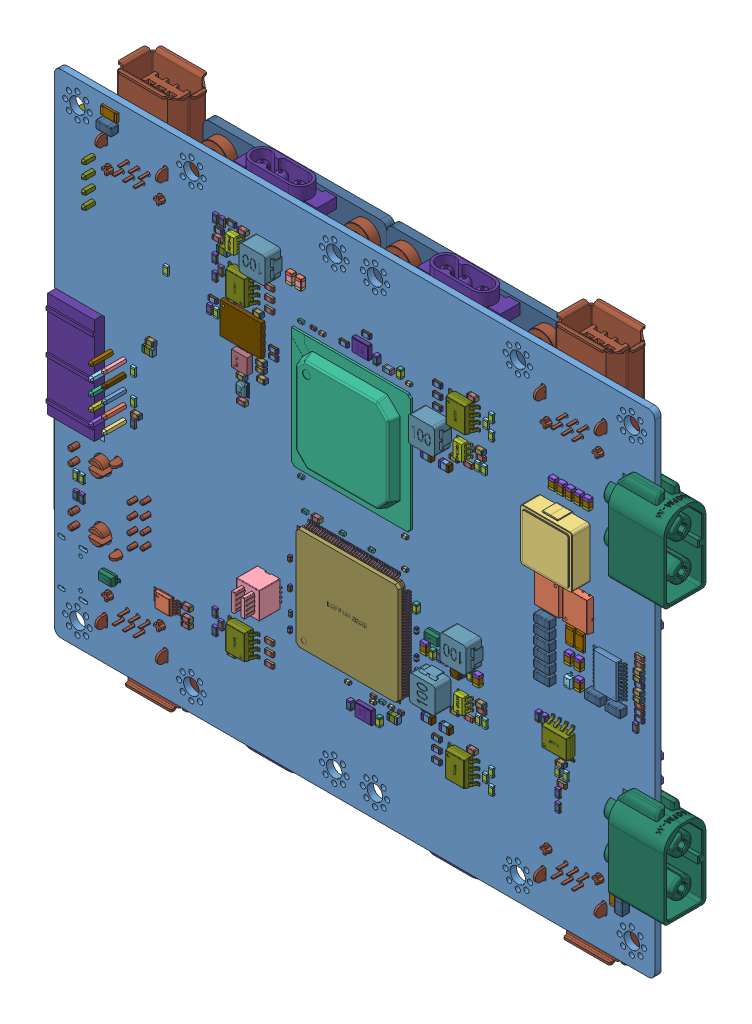
SolidWorks assembly Mother  Board, configuration 默认. Lengths in mm. (continued)
Components (placement in the parent): (continued)
- Mother  Board.step-1: Mother  Board.step [默认] at origin size (122.6 102.08 21) (continued)
  - Free-Models.step-1: Free-Models.step [默认] at origin size (70.87 98.07 8.62) (continued)
    - Driver_Board.step-2: Driver_Board.step [默认] at (84.963 86.106 -6.2) x (-1 0 0) z (0 0 1) size (35.43 49.03 8.62) (continued)
      - C19-1.step-1: C19-1.step [默认] at origin size (0.8 1.6 0.8) (continued)
        - 6547517776.step-1: 6547517776.step [默认] at (25.7809 37.7191 0) x (0 1 0) z (0 0 1) size (1.6 0.8 0.8) (continued)
          - Terminal-24.step-1: Terminal-24.step [默认] at (-0.8 -0.4 0) size (1.6 0.8 0.8) (continued)
            - Open_CASCADE_STEP_translator_6.8_47.1.2-105.step-1: Open_CASCADE_STEP_translator_6.8_47.1.2-105.step [默认] at origin size (0.3 0.8 0.8)
          - Mid_Body-12.step-1: Mid_Body-12.step [默认] at (-0.8 -0.4 0) size (1 0.8 0.8)
            - Open_CASCADE_STEP_translator_6.8_47.2.1-106.step-1: Open_CASCADE_STEP_translator_6.8_47.2.1-106.step [默认] at origin size (1 0.8 0.8)
      - C18-1.step-1: C18-1.step [默认] at origin size (0.8 1.6 0.8)
        - 6547517776.step-1: 6547517776.step [默认] at (24.6379 37.7191 0) x (0 1 0) z (0 0 1) size (1.6 0.8 0.8)
          - Terminal-24.step-1: Terminal-24.step [默认] at (-0.8 -0.4 0) size (1.6 0.8 0.8)
            - Open_CASCADE_STEP_translator_6.8_47.1.1-104.step-1: Open_CASCADE_STEP_translator_6.8_47.1.1-104.step [默认] at origin size (0.3 0.8 0.8)
            - Open_CASCADE_STEP_translator_6.8_47.1.2-105.step-1: Open_CASCADE_STEP_translator_6.8_47.1.2-105.step [默认] at origin size (0.3 0.8 0.8)
          - Mid_Body-12.step-1: Mid_Body-12.step [默认] at (-0.8 -0.4 0) size (1 0.8 0.8)
            - Open_CASCADE_STEP_translator_6.8_47.2.1-106.step-1: Open_CASCADE_STEP_translator_6.8_47.2.1-106.step [默认] at origin size (1 0.8 0.8)
      - C17-1.step-1: C17-1.step [默认] at origin size (1.6 0.8 0.8)
        - 6547515616.step-1: 6547515616.step [默认] at (13.7159 12.9539 0) x (-1 0 0) z (0 0 1) size (1.6 0.8 0.8)
          - Terminal-22.step-1: Terminal-22.step [默认] at (-0.8 -0.4 0) size (1.6 0.8 0.8)
            - Open_CASCADE_STEP_translator_6.8_47.1.1-85.step-1: Open_CASCADE_STEP_translator_6.8_47.1.1-85.step [默认] at origin size (0.3 0.8 0.8)
            - Open_CASCADE_STEP_translator_6.8_47.1.2-86.step-1: Open_CASCADE_STEP_translator_6.8_47.1.2-86.step [默认] at origin size (0.3 0.8 0.8)
          - Mid_Body-10.step-1: Mid_Body-10.step [默认] at (-0.8 -0.4 0) size (1 0.8 0.8)
            - Open_CASCADE_STEP_translator_6.8_47.2.1-87.step-1: Open_CASCADE_STEP_translator_6.8_47.2.1-87.step [默认] at origin size (1 0.8 0.8)
      - C16-1.step-1: C16-1.step [默认] at origin size (0.8 1.6 0.8)
        - 6547516096.step-1: 6547516096.step [默认] at (25.7811 22.2249 0) x (0 -1 0) z (0 0 1) size (1.6 0.8 0.8)
          - Terminal-23.step-1: Terminal-23.step [默认] at (-0.8 -0.4 0) size (1.6 0.8 0.8)
            - Open_CASCADE_STEP_translator_6.8_47.1.1-98.step-1: Open_CASCADE_STEP_translator_6.8_47.1.1-98.step [默认] at origin size (0.3 0.8 0.8)
            - Open_CASCADE_STEP_translator_6.8_47.1.2-99.step-1: Open_CASCADE_STEP_translator_6.8_47.1.2-99.step [默认] at origin size (0.3 0.8 0.8)
          - Mid_Body-11.step-1: Mid_Body-11.step [默认] at (-0.8 -0.4 0) size (1 0.8 0.8)
            - Open_CASCADE_STEP_translator_6.8_47.2.1-100.step-1: Open_CASCADE_STEP_translator_6.8_47.2.1-100.step [默认] at origin size (1 0.8 0.8)
      - C15-1.step-1: C15-1.step [默认] at origin size (0.8 1.6 0.8)
        - 6547517776.step-1: 6547517776.step [默认] at (23.8759 25.6541 0) x (0 1 0) z (0 0 1) size (1.6 0.8 0.8)
          - Terminal-24.step-1: Terminal-24.step [默认] at (-0.8 -0.4 0) size (1.6 0.8 0.8)
            - Open_CASCADE_STEP_translator_6.8_47.1.1-104.step-1: Open_CASCADE_STEP_translator_6.8_47.1.1-104.step [默认] at origin size (0.3 0.8 0.8)
            - Open_CASCADE_STEP_translator_6.8_47.1.2-105.step-1: Open_CASCADE_STEP_translator_6.8_47.1.2-105.step [默认] at origin size (0.3 0.8 0.8)
          - Mid_Body-12.step-1: Mid_Body-12.step [默认] at (-0.8 -0.4 0) size (1 0.8 0.8)
            - Open_CASCADE_STEP_translator_6.8_47.2.1-106.step-1: Open_CASCADE_STEP_translator_6.8_47.2.1-106.step [默认] at origin size (1 0.8 0.8)
      - C14-1.step-1: C14-1.step [默认] at origin size (2.01 1.25 0.94)
        - 6547513136.step-1: 6547513136.step [默认] at (13.7383 23.4725 0) x (-1 0 0) z (0 0 1) size (2.01 1.25 0.94)
          - Fillet1-95.step-1: Fillet1-95.step [默认] at origin size (0.5 1.25 0.94)
          - Fillet2-96.step-1: Fillet2-96.step [默认] at origin size (0.5 1.25 0.94)
          - body2-97.step-1: body2-97.step [默认] at origin size (1.01 1.22 0.92)
      - C13-1.step-1: C13-1.step [默认] at origin size (0.8 1.6 0.8)
        - 6547516096.step-1: 6547516096.step [默认] at (10.8175 24.7425 0) x (0 -1 0) z (0 0 1) size (1.6 0.8 0.8)
          - Terminal-23.step-1: Terminal-23.step [默认] at (-0.8 -0.4 0) size (1.6 0.8 0.8)
            - Open_CASCADE_STEP_translator_6.8_47.1.1-98.step-1: Open_CASCADE_STEP_translator_6.8_47.1.1-98.step [默认] at origin size (0.3 0.8 0.8)
            - Open_CASCADE_STEP_translator_6.8_47.1.2-99.step-1: Open_CASCADE_STEP_translator_6.8_47.1.2-99.step [默认] at origin size (0.3 0.8 0.8)
          - Mid_Body-11.step-1: Mid_Body-11.step [默认] at (-0.8 -0.4 0) size (1 0.8 0.8)
            - Open_CASCADE_STEP_translator_6.8_47.2.1-100.step-1: Open_CASCADE_STEP_translator_6.8_47.2.1-100.step [默认] at origin size (1 0.8 0.8)
      - C12-1.step-1: C12-1.step [默认] at origin size (1.25 2.01 0.94)
        - 6547514896.step-1: 6547514896.step [默认] at (16.4053 31.0126 0) x (0 1 0) z (0 0 1) size (2.01 1.25 0.94)
          - Fillet1-101.step-1: Fillet1-101.step [默认] at origin size (0.5 1.25 0.94)
          - Fillet2-102.step-1: Fillet2-102.step [默认] at origin size (0.5 1.25 0.94)
          - body2-103.step-1: body2-103.step [默认] at origin size (1.01 1.22 0.92)
      - C11-1.step-1: C11-1.step [默认] at origin size (1.6 0.8 0.8)
        - 6547515616.step-1: 6547515616.step [默认] at (27.6859 22.8599 0) x (-1 0 0) z (0 0 1) size (1.6 0.8 0.8)
          - Terminal-22.step-1: Terminal-22.step [默认] at (-0.8 -0.4 0) size (1.6 0.8 0.8)
            - Open_CASCADE_STEP_translator_6.8_47.1.1-85.step-1: Open_CASCADE_STEP_translator_6.8_47.1.1-85.step [默认] at origin size (0.3 0.8 0.8)
            - Open_CASCADE_STEP_translator_6.8_47.1.2-86.step-1: Open_CASCADE_STEP_translator_6.8_47.1.2-86.step [默认] at origin size (0.3 0.8 0.8)
          - Mid_Body-10.step-1: Mid_Body-10.step [默认] at (-0.8 -0.4 0) size (1 0.8 0.8)
            - Open_CASCADE_STEP_translator_6.8_47.2.1-87.step-1: Open_CASCADE_STEP_translator_6.8_47.2.1-87.step [默认] at origin size (1 0.8 0.8)
      - C10-1.step-1: C10-1.step [默认] at origin size (0.8 1.6 0.8)
        - 6547517776.step-1: 6547517776.step [默认] at (-3.1751 37.7191 0) x (0 1 0) z (0 0 1) size (1.6 0.8 0.8)
          - Terminal-24.step-1: Terminal-24.step [默认] at (-0.8 -0.4 0) size (1.6 0.8 0.8)
            - Open_CASCADE_STEP_translator_6.8_47.1.1-104.step-1: Open_CASCADE_STEP_translator_6.8_47.1.1-104.step [默认] at origin size (0.3 0.8 0.8)
            - Open_CASCADE_STEP_translator_6.8_47.1.2-105.step-1: Open_CASCADE_STEP_translator_6.8_47.1.2-105.step [默认] at origin size (0.3 0.8 0.8)
          - Mid_Body-12.step-1: Mid_Body-12.step [默认] at (-0.8 -0.4 0) size (1 0.8 0.8)
            - Open_CASCADE_STEP_translator_6.8_47.2.1-106.step-1: Open_CASCADE_STEP_translator_6.8_47.2.1-106.step [默认] at origin size (1 0.8 0.8)
      - C9-1.step-1: C9-1.step [默认] at origin size (0.8 1.6 0.8)
        - 6547516096.step-1: 6547516096.step [默认] at (-3.1749 22.2249 0) x (0 -1 0) z (0 0 1) size (1.6 0.8 0.8)
          - Terminal-23.step-1: Terminal-23.step [默认] at (-0.8 -0.4 0) size (1.6 0.8 0.8)
            - Open_CASCADE_STEP_translator_6.8_47.1.1-98.step-1: Open_CASCADE_STEP_translator_6.8_47.1.1-98.step [默认] at origin size (0.3 0.8 0.8)
            - Open_CASCADE_STEP_translator_6.8_47.1.2-99.step-1: Open_CASCADE_STEP_translator_6.8_47.1.2-99.step [默认] at origin size (0.3 0.8 0.8)
          - Mid_Body-11.step-1: Mid_Body-11.step [默认] at (-0.8 -0.4 0) size (1 0.8 0.8)
            - Open_CASCADE_STEP_translator_6.8_47.2.1-100.step-1: Open_CASCADE_STEP_translator_6.8_47.2.1-100.step [默认] at origin size (1 0.8 0.8)
      - C8-1.step-1: C8-1.step [默认] at origin size (1.6 0.8 0.8)
        - 6547515616.step-1: 6547515616.step [默认] at (1.1429 16.5099 0) x (-1 0 0) z (0 0 1) size (1.6 0.8 0.8)
          - Terminal-22.step-1: Terminal-22.step [默认] at (-0.8 -0.4 0) size (1.6 0.8 0.8)
            - Open_CASCADE_STEP_translator_6.8_47.1.1-85.step-1: Open_CASCADE_STEP_translator_6.8_47.1.1-85.step [默认] at origin size (0.3 0.8 0.8)
            - Open_CASCADE_STEP_translator_6.8_47.1.2-86.step-1: Open_CASCADE_STEP_translator_6.8_47.1.2-86.step [默认] at origin size (0.3 0.8 0.8)
          - Mid_Body-10.step-1: Mid_Body-10.step [默认] at (-0.8 -0.4 0) size (1 0.8 0.8)
            - Open_CASCADE_STEP_translator_6.8_47.2.1-87.step-1: Open_CASCADE_STEP_translator_6.8_47.2.1-87.step [默认] at origin size (1 0.8 0.8)
      - C7-1.step-1: C7-1.step [默认] at origin size (0.8 1.6 0.8)
        - 6547516096.step-1: 6547516096.step [默认] at (-2.0319 22.2249 0) x (0 -1 0) z (0 0 1) size (1.6 0.8 0.8)
          - Terminal-23.step-1: Terminal-23.step [默认] at (-0.8 -0.4 0) size (1.6 0.8 0.8)
            - Open_CASCADE_STEP_translator_6.8_47.1.1-98.step-1: Open_CASCADE_STEP_translator_6.8_47.1.1-98.step [默认] at origin size (0.3 0.8 0.8)
            - Open_CASCADE_STEP_translator_6.8_47.1.2-99.step-1: Open_CASCADE_STEP_translator_6.8_47.1.2-99.step [默认] at origin size (0.3 0.8 0.8)
          - Mid_Body-11.step-1: Mid_Body-11.step [默认] at (-0.8 -0.4 0) size (1 0.8 0.8)
            - Open_CASCADE_STEP_translator_6.8_47.2.1-100.step-1: Open_CASCADE_STEP_translator_6.8_47.2.1-100.step [默认] at origin size (1 0.8 0.8)
      - C6-1.step-1: C6-1.step [默认] at origin size (0.8 1.6 0.8)
        - 6547517776.step-1: 6547517776.step [默认] at (-2.0321 37.7191 0) x (0 1 0) z (0 0 1) size (1.6 0.8 0.8)
          - Terminal-24.step-1: Terminal-24.step [默认] at (-0.8 -0.4 0) size (1.6 0.8 0.8)
            - Open_CASCADE_STEP_translator_6.8_47.1.1-104.step-1: Open_CASCADE_STEP_translator_6.8_47.1.1-104.step [默认] at origin size (0.3 0.8 0.8)
            - Open_CASCADE_STEP_translator_6.8_47.1.2-105.step-1: Open_CASCADE_STEP_translator_6.8_47.1.2-105.step [默认] at origin size (0.3 0.8 0.8)
          - Mid_Body-12.step-1: Mid_Body-12.step [默认] at (-0.8 -0.4 0) size (1 0.8 0.8)
            - Open_CASCADE_STEP_translator_6.8_47.2.1-106.step-1: Open_CASCADE_STEP_translator_6.8_47.2.1-106.step [默认] at origin size (1 0.8 0.8)
      - C5-1.step-1: C5-1.step [默认] at origin size (1.6 0.8 0.8)
        - 6547515616.step-1: 6547515616.step [默认] at (2.7939 10.6679 0) x (-1 0 0) z (0 0 1) size (1.6 0.8 0.8)
          - Terminal-22.step-1: Terminal-22.step [默认] at (-0.8 -0.4 0) size (1.6 0.8 0.8)
            - Open_CASCADE_STEP_translator_6.8_47.1.1-85.step-1: Open_CASCADE_STEP_translator_6.8_47.1.1-85.step [默认] at origin size (0.3 0.8 0.8)
            - Open_CASCADE_STEP_translator_6.8_47.1.2-86.step-1: Open_CASCADE_STEP_translator_6.8_47.1.2-86.step [默认] at origin size (0.3 0.8 0.8)
          - Mid_Body-10.step-1: Mid_Body-10.step [默认] at (-0.8 -0.4 0) size (1 0.8 0.8)
            - Open_CASCADE_STEP_translator_6.8_47.2.1-87.step-1: Open_CASCADE_STEP_translator_6.8_47.2.1-87.step [默认] at origin size (1 0.8 0.8)
      - C4-1.step-1: C4-1.step [默认] at origin size (1.6 0.8 0.8)
        - 6547515616.step-1: 6547515616.step [默认] at (-0.1271 22.8599 0) x (-1 0 0) z (0 0 1) size (1.6 0.8 0.8)
          - Terminal-22.step-1: Terminal-22.step [默认] at (-0.8 -0.4 0) size (1.6 0.8 0.8)
            - Open_CASCADE_STEP_translator_6.8_47.1.1-85.step-1: Open_CASCADE_STEP_translator_6.8_47.1.1-85.step [默认] at origin size (0.3 0.8 0.8)
            - Open_CASCADE_STEP_translator_6.8_47.1.2-86.step-1: Open_CASCADE_STEP_translator_6.8_47.1.2-86.step [默认] at origin size (0.3 0.8 0.8)
          - Mid_Body-10.step-1: Mid_Body-10.step [默认] at (-0.8 -0.4 0) size (1 0.8 0.8)
            - Open_CASCADE_STEP_translator_6.8_47.2.1-87.step-1: Open_CASCADE_STEP_translator_6.8_47.2.1-87.step [默认] at origin size (1 0.8 0.8)
      - C3-1.step-1: C3-1.step [默认] at origin size (2.01 1.25 0.94)
        - 6547513136.step-1: 6547513136.step [默认] at (6.6263 23.4725 0) x (-1 0 0) z (0 0 1) size (2.01 1.25 0.94)
          - Fillet1-95.step-1: Fillet1-95.step [默认] at origin size (0.5 1.25 0.94)
          - Fillet2-96.step-1: Fillet2-96.step [默认] at origin size (0.5 1.25 0.94)
          - body2-97.step-1: body2-97.step [默认] at origin size (1.01 1.22 0.92)
      - C2-1.step-1: C2-1.step [默认] at origin size (0.8 1.6 0.8)
        - 6547516096.step-1: 6547516096.step [默认] at (3.7055 24.7425 0) x (0 -1 0) z (0 0 1) size (1.6 0.8 0.8)
          - Terminal-23.step-1: Terminal-23.step [默认] at (-0.8 -0.4 0) size (1.6 0.8 0.8)
            - Open_CASCADE_STEP_translator_6.8_47.1.1-98.step-1: Open_CASCADE_STEP_translator_6.8_47.1.1-98.step [默认] at origin size (0.3 0.8 0.8)
            - Open_CASCADE_STEP_translator_6.8_47.1.2-99.step-1: Open_CASCADE_STEP_translator_6.8_47.1.2-99.step [默认] at origin size (0.3 0.8 0.8)
          - Mid_Body-11.step-1: Mid_Body-11.step [默认] at (-0.8 -0.4 0) size (1 0.8 0.8)
            - Open_CASCADE_STEP_translator_6.8_47.2.1-100.step-1: Open_CASCADE_STEP_translator_6.8_47.2.1-100.step [默认] at origin size (1 0.8 0.8)
      - C1.step-1: C1.step [默认] at origin size (1.25 2.01 0.94)
        - 6547514896.step-1: 6547514896.step [默认] at (9.2933 31.0126 0) x (0 1 0) z (0 0 1) size (2.01 1.25 0.94)
          - Fillet1-101.step-1: Fillet1-101.step [默认] at origin size (0.5 1.25 0.94)
          - Fillet2-102.step-1: Fillet2-102.step [默认] at origin size (0.5 1.25 0.94)
          - body2-103.step-1: body2-103.step [默认] at origin size (1.01 1.22 0.92)
    - Driver_Board.step-3: Driver_Board.step [默认] at (57.3933 0 -6.2) x (1 0 0) z (0 0 1) size (35.43 49.03 8.62)
      - Board-1.step-1: Board-1.step [默认] at origin size (35.43 46.99 1.62)
        - Open_CASCADE_STEP_translator_6.8_2.1.1.step-1: Open_CASCADE_STEP_translator_6.8_2.1.1.step [默认] at (0 0 -1.6164) size (35.43 46.99 1.62)
      - R25-1.step-1: R25-1.step [默认] at origin size (0.8 1.6 0.45)
        - 6547515376.step-1: 6547515376.step [默认] at (20.6304 35.5601 0) x (0 1 0) z (0 0 1) size (1.6 0.8 0.45)
          - Terminal-19.step-1: Terminal-19.step [默认] at (-0.8 -0.4 0) size (0.3 0.8 0.45)
            - Open_CASCADE_STEP_translator_6.8_21.2.1-76.step-1: Open_CASCADE_STEP_translator_6.8_21.2.1-76.step [默认] at origin size (0.3 0.8 0.45)
          - Terminal-19.step-2: Terminal-19.step [默认] at (0.8 0.4 0) x (-1 0 0) z (0 0 1) size (0.3 0.8 0.45)
            - Open_CASCADE_STEP_translator_6.8_21.2.1-76.step-1: Open_CASCADE_STEP_translator_6.8_21.2.1-76.step [默认] at origin size (0.3 0.8 0.45)
          - Mid_Body-77.step-1: Mid_Body-77.step [默认] at (-0.8 -0.4 0) size (1.51 0.8 0.36)
          - Mark-78.step-1: Mark-78.step [默认] at (-0.5 -0.4 0.405) size (1 0.8 0.05)
      - R24-1.step-1: R24-1.step [默认] at origin size (1.6 0.8 0.45)
        - 6547516336.step-1: 6547516336.step [默认] at (12.6999 34.9249 0) x (-1 0 0) z (0 0 1) size (1.6 0.8 0.45)
          - Terminal-20.step-1: Terminal-20.step [默认] at (-0.8 -0.4 0) size (0.3 0.8 0.45)
            - Open_CASCADE_STEP_translator_6.8_21.2.1-79.step-1: Open_CASCADE_STEP_translator_6.8_21.2.1-79.step [默认] at origin size (0.3 0.8 0.45)
          - Terminal-20.step-2: Terminal-20.step [默认] at (0.8 0.4 0) x (-1 0 0) z (0 0 1) size (0.3 0.8 0.45)
            - Open_CASCADE_STEP_translator_6.8_21.2.1-79.step-1: Open_CASCADE_STEP_translator_6.8_21.2.1-79.step [默认] at origin size (0.3 0.8 0.45)
          - Mid_Body-80.step-1: Mid_Body-80.step [默认] at (-0.8 -0.4 0) size (1.51 0.8 0.36)
          - Mark-81.step-1: Mark-81.step [默认] at (-0.5 -0.4 0.405) size (1 0.8 0.05)
      - R23-1.step-1: R23-1.step [默认] at origin size (1.6 0.8 0.45)
        - 6547516336.step-1: 6547516336.step [默认] at (5.5879 33.6549 0) x (-1 0 0) z (0 0 1) size (1.6 0.8 0.45)
          - Terminal-20.step-1: Terminal-20.step [默认] at (-0.8 -0.4 0) size (0.3 0.8 0.45)
            - Open_CASCADE_STEP_translator_6.8_21.2.1-79.step-1: Open_CASCADE_STEP_translator_6.8_21.2.1-79.step [默认] at origin size (0.3 0.8 0.45)
          - Terminal-20.step-2: Terminal-20.step [默认] at (0.8 0.4 0) x (-1 0 0) z (0 0 1) size (0.3 0.8 0.45)
            - Open_CASCADE_STEP_translator_6.8_21.2.1-79.step-1: Open_CASCADE_STEP_translator_6.8_21.2.1-79.step [默认] at origin size (0.3 0.8 0.45)
          - Mid_Body-80.step-1: Mid_Body-80.step [默认] at (-0.8 -0.4 0) size (1.51 0.8 0.36)
          - Mark-81.step-1: Mark-81.step [默认] at (-0.5 -0.4 0.405) size (1 0.8 0.05)
      - JP1.step-1: JP1.step [默认] at origin size (16.01 14.49 6.96)
        - User_Library-MR30PW-M.step-1: User_Library-MR30PW-M.step [默认] at (13.7158 -5.9802 2.75) x (1 0 0) z (0 0 1) size (16.01 14.49 6.96)
      - R18-1.step-1: R18-1.step [默认] at origin size (0.8 1.6 0.45)
        - 6547515376.step-1: 6547515376.step [默认] at (22.9869 34.4171 0) x (0 1 0) z (0 0 1) size (1.6 0.8 0.45)
          - Terminal-19.step-1: Terminal-19.step [默认] at (-0.8 -0.4 0) size (0.3 0.8 0.45)
            - Open_CASCADE_STEP_translator_6.8_21.2.1-76.step-1: Open_CASCADE_STEP_translator_6.8_21.2.1-76.step [默认] at origin size (0.3 0.8 0.45)
          - Terminal-19.step-2: Terminal-19.step [默认] at (0.8 0.4 0) x (-1 0 0) z (0 0 1) size (0.3 0.8 0.45)
            - Open_CASCADE_STEP_translator_6.8_21.2.1-76.step-1: Open_CASCADE_STEP_translator_6.8_21.2.1-76.step [默认] at origin size (0.3 0.8 0.45)
          - Mid_Body-77.step-1: Mid_Body-77.step [默认] at (-0.8 -0.4 0) size (1.51 0.8 0.36)
          - Mark-78.step-1: Mark-78.step [默认] at (-0.5 -0.4 0.405) size (1 0.8 0.05)
      - R17-1.step-1: R17-1.step [默认] at origin size (0.8 1.6 0.45)
        - 6547515376.step-1: 6547515376.step [默认] at (21.8663 34.3947 0) x (0 1 0) z (0 0 1) size (1.6 0.8 0.45)
          - Terminal-19.step-1: Terminal-19.step [默认] at (-0.8 -0.4 0) size (0.3 0.8 0.45)
            - Open_CASCADE_STEP_translator_6.8_21.2.1-76.step-1: Open_CASCADE_STEP_translator_6.8_21.2.1-76.step [默认] at origin size (0.3 0.8 0.45)
          - Terminal-19.step-2: Terminal-19.step [默认] at (0.8 0.4 0) x (-1 0 0) z (0 0 1) size (0.3 0.8 0.45)
            - Open_CASCADE_STEP_translator_6.8_21.2.1-76.step-1: Open_CASCADE_STEP_translator_6.8_21.2.1-76.step [默认] at origin size (0.3 0.8 0.45)
          - Mid_Body-77.step-1: Mid_Body-77.step [默认] at (-0.8 -0.4 0) size (1.51 0.8 0.36)
          - Mark-78.step-1: Mark-78.step [默认] at (-0.5 -0.4 0.405) size (1 0.8 0.05)
      - R16-1.step-1: R16-1.step [默认] at origin size (1.6 0.8 0.45)
        - 6547506496.step-1: 6547506496.step [默认] at (16.6371 33.6551 0) x (1 0 0) z (0 0 1) size (1.6 0.8 0.45)
          - Terminal-21.step-1: Terminal-21.step [默认] at (-0.8 -0.4 0) size (0.3 0.8 0.45)
            - Open_CASCADE_STEP_translator_6.8_21.2.1-82.step-1: Open_CASCADE_STEP_translator_6.8_21.2.1-82.step [默认] at origin size (0.3 0.8 0.45)
          - Terminal-21.step-2: Terminal-21.step [默认] at (0.8 0.4 0) x (-1 0 0) z (0 0 1) size (0.3 0.8 0.45)
            - Open_CASCADE_STEP_translator_6.8_21.2.1-82.step-1: Open_CASCADE_STEP_translator_6.8_21.2.1-82.step [默认] at origin size (0.3 0.8 0.45)
          - Mid_Body-83.step-1: Mid_Body-83.step [默认] at (-0.8 -0.4 0) size (1.51 0.8 0.36)
          - Mark-84.step-1: Mark-84.step [默认] at (-0.5 -0.4 0.405) size (1 0.8 0.05)
      - R15-1.step-1: R15-1.step [默认] at origin size (0.8 1.6 0.45)
        - 6547515376.step-1: 6547515376.step [默认] at (14.7319 34.2901 0) x (0 1 0) z (0 0 1) size (1.6 0.8 0.45)
          - Terminal-19.step-1: Terminal-19.step [默认] at (-0.8 -0.4 0) size (0.3 0.8 0.45)
            - Open_CASCADE_STEP_translator_6.8_21.2.1-76.step-1: Open_CASCADE_STEP_translator_6.8_21.2.1-76.step [默认] at origin size (0.3 0.8 0.45)
          - Terminal-19.step-2: Terminal-19.step [默认] at (0.8 0.4 0) x (-1 0 0) z (0 0 1) size (0.3 0.8 0.45)
            - Open_CASCADE_STEP_translator_6.8_21.2.1-76.step-1: Open_CASCADE_STEP_translator_6.8_21.2.1-76.step [默认] at origin size (0.3 0.8 0.45)
          - Mid_Body-77.step-1: Mid_Body-77.step [默认] at (-0.8 -0.4 0) size (1.51 0.8 0.36)
          - Mark-78.step-1: Mark-78.step [默认] at (-0.5 -0.4 0.405) size (1 0.8 0.05)
      - R13-1.step-1: R13-1.step [默认] at origin size (1.6 0.8 0.45)
        - 6547506496.step-1: 6547506496.step [默认] at (9.5251 33.6551 0) x (1 0 0) z (0 0 1) size (1.6 0.8 0.45)
          - Terminal-21.step-1: Terminal-21.step [默认] at (-0.8 -0.4 0) size (0.3 0.8 0.45)
            - Open_CASCADE_STEP_translator_6.8_21.2.1-82.step-1: Open_CASCADE_STEP_translator_6.8_21.2.1-82.step [默认] at origin size (0.3 0.8 0.45)
          - Terminal-21.step-2: Terminal-21.step [默认] at (0.8 0.4 0) x (-1 0 0) z (0 0 1) size (0.3 0.8 0.45)
            - Open_CASCADE_STEP_translator_6.8_21.2.1-82.step-1: Open_CASCADE_STEP_translator_6.8_21.2.1-82.step [默认] at origin size (0.3 0.8 0.45)
          - Mid_Body-83.step-1: Mid_Body-83.step [默认] at (-0.8 -0.4 0) size (1.51 0.8 0.36)
          - Mark-84.step-1: Mark-84.step [默认] at (-0.5 -0.4 0.405) size (1 0.8 0.05)
      - R11-1.step-1: R11-1.step [默认] at origin size (0.8 1.6 0.45)
        - 6547515376.step-1: 6547515376.step [默认] at (7.6423 34.2901 0) x (0 1 0) z (0 0 1) size (1.6 0.8 0.45)
          - Terminal-19.step-1: Terminal-19.step [默认] at (-0.8 -0.4 0) size (0.3 0.8 0.45)
            - Open_CASCADE_STEP_translator_6.8_21.2.1-76.step-1: Open_CASCADE_STEP_translator_6.8_21.2.1-76.step [默认] at origin size (0.3 0.8 0.45)
          - Terminal-19.step-2: Terminal-19.step [默认] at (0.8 0.4 0) x (-1 0 0) z (0 0 1) size (0.3 0.8 0.45)
            - Open_CASCADE_STEP_translator_6.8_21.2.1-76.step-1: Open_CASCADE_STEP_translator_6.8_21.2.1-76.step [默认] at origin size (0.3 0.8 0.45)
          - Mid_Body-77.step-1: Mid_Body-77.step [默认] at (-0.8 -0.4 0) size (1.51 0.8 0.36)
          - Mark-78.step-1: Mark-78.step [默认] at (-0.5 -0.4 0.405) size (1 0.8 0.05)
      - C23-1.step-1: C23-1.step [默认] at origin size (1.6 0.8 0.8)
        - 6547515616.step-1: 6547515616.step [默认] at (19.8684 33.6676 0) x (-1 0 0) z (0 0 1) size (1.6 0.8 0.8)
          - Terminal-22.step-1: Terminal-22.step [默认] at (-0.8 -0.4 0) size (1.6 0.8 0.8)
            - Open_CASCADE_STEP_translator_6.8_47.1.1-85.step-1: Open_CASCADE_STEP_translator_6.8_47.1.1-85.step [默认] at origin size (0.3 0.8 0.8)
            - Open_CASCADE_STEP_translator_6.8_47.1.2-86.step-1: Open_CASCADE_STEP_translator_6.8_47.1.2-86.step [默认] at origin size (0.3 0.8 0.8)
          - Mid_Body-10.step-1: Mid_Body-10.step [默认] at (-0.8 -0.4 0) size (1 0.8 0.8)
            - Open_CASCADE_STEP_translator_6.8_47.2.1-87.step-1: Open_CASCADE_STEP_translator_6.8_47.2.1-87.step [默认] at origin size (1 0.8 0.8)
      - C22-1.step-1: C22-1.step [默认] at origin size (1.6 0.8 0.8)
        - 6547515616.step-1: 6547515616.step [默认] at (12.6999 33.6549 0) x (-1 0 0) z (0 0 1) size (1.6 0.8 0.8)
          - Terminal-22.step-1: Terminal-22.step [默认] at (-0.8 -0.4 0) size (1.6 0.8 0.8)
            - Open_CASCADE_STEP_translator_6.8_47.1.1-85.step-1: Open_CASCADE_STEP_translator_6.8_47.1.1-85.step [默认] at origin size (0.3 0.8 0.8)
            - Open_CASCADE_STEP_translator_6.8_47.1.2-86.step-1: Open_CASCADE_STEP_translator_6.8_47.1.2-86.step [默认] at origin size (0.3 0.8 0.8)
          - Mid_Body-10.step-1: Mid_Body-10.step [默认] at (-0.8 -0.4 0) size (1 0.8 0.8)
            - Open_CASCADE_STEP_translator_6.8_47.2.1-87.step-1: Open_CASCADE_STEP_translator_6.8_47.2.1-87.step [默认] at origin size (1 0.8 0.8)
      - C21-1.step-1: C21-1.step [默认] at origin size (1.6 0.8 0.8)
        - 6547515616.step-1: 6547515616.step [默认] at (5.6103 34.9025 0) x (-1 0 0) z (0 0 1) size (1.6 0.8 0.8)
          - Terminal-22.step-1: Terminal-22.step [默认] at (-0.8 -0.4 0) size (1.6 0.8 0.8)
            - Open_CASCADE_STEP_translator_6.8_47.1.1-85.step-1: Open_CASCADE_STEP_translator_6.8_47.1.1-85.step [默认] at origin size (0.3 0.8 0.8)
            - Open_CASCADE_STEP_translator_6.8_47.1.2-86.step-1: Open_CASCADE_STEP_translator_6.8_47.1.2-86.step [默认] at origin size (0.3 0.8 0.8)
          - Mid_Body-10.step-1: Mid_Body-10.step [默认] at (-0.8 -0.4 0) size (1 0.8 0.8)
            - Open_CASCADE_STEP_translator_6.8_47.2.1-87.step-1: Open_CASCADE_STEP_translator_6.8_47.2.1-87.step [默认] at origin size (1 0.8 0.8)
      - U5-1.step-1: U5-1.step [默认] at origin size (5.9 11.5 2.7)
        - SO8_W.step-1: SO8_W.step [默认] at (27.6859 29.9721 0.381) x (0 1 0) z (0 0 1) size (11.5 5.9 2.7)
      - U4-1.step-1: U4-1.step [默认] at origin size (5.9 11.5 2.7)
        - SO8_W.step-1: SO8_W.step [默认] at (-0.1271 29.9721 0.381) x (0 1 0) z (0 0 1) size (11.5 5.9 2.7)
      - U3-1.step-1: U3-1.step [默认] at origin size (5 6.01 1.9)
        - SOP8-1.step-1: SOP8-1.step [默认] at (19.9615 29.5285 0) x (0 -1 0) z (0 0 1) size (6.01 5 1.9)
          - LOGO_-88.step-1: LOGO_-88.step [默认] at (0.0116 0 0.095) x (0 -1 0) z (0 0 -1) size (1.5 1.73 0.01)
          - SOP8-89.step-1: SOP8-89.step [默认] at origin size (6.01 5 1.9)
      - U2-1.step-1: U2-1.step [默认] at origin size (5 6.01 1.9)
        - SOP8-1.step-1: SOP8-1.step [默认] at (12.8495 29.5285 0) x (0 -1 0) z (0 0 1) size (6.01 5 1.9)
          - LOGO_-88.step-1: LOGO_-88.step [默认] at (0.0116 0 0.095) x (0 -1 0) z (0 0 -1) size (1.5 1.73 0.01)
          - SOP8-89.step-1: SOP8-89.step [默认] at origin size (6.01 5 1.9)
      - U1.step-1: U1.step [默认] at origin size (5 6.01 1.9)
        - SOP8-1.step-1: SOP8-1.step [默认] at (5.7375 29.5285 0) x (0 -1 0) z (0 0 1) size (6.01 5 1.9)
          - LOGO_-88.step-1: LOGO_-88.step [默认] at (0.0116 0 0.095) x (0 -1 0) z (0 0 -1) size (1.5 1.73 0.01)
          - SOP8-89.step-1: SOP8-89.step [默认] at origin size (6.01 5 1.9)
      - RS2-1.step-1: RS2-1.step [默认] at origin size (3.1 1.55 0.47)
        - User_Library-R1206-90.step-1: User_Library-R1206-90.step [默认] at (23.7489 17.5261 -1.6164) x (-1 0 0) z (0 0 -1) size (3.1 1.55 0.47)
      - RS1-1.step-1: RS1-1.step [默认] at origin size (3.1 1.55 0.47)
        - User_Library-R1206-90.step-1: User_Library-R1206-90.step [默认] at (-0.1271 18.1611 -1.6164) x (-1 0 0) z (0 0 -1) size (3.1 1.55 0.47)
      - R22-1.step-1: R22-1.step [默认] at origin size (1.6 0.8 0.45)
        - 6547506496.step-1: 6547506496.step [默认] at (22.9871 17.7801 0) x (1 0 0) z (0 0 1) size (1.6 0.8 0.45)
          - Terminal-21.step-1: Terminal-21.step [默认] at (-0.8 -0.4 0) size (0.3 0.8 0.45)
            - Open_CASCADE_STEP_translator_6.8_21.2.1-82.step-1: Open_CASCADE_STEP_translator_6.8_21.2.1-82.step [默认] at origin size (0.3 0.8 0.45)
          - Terminal-21.step-2: Terminal-21.step [默认] at (0.8 0.4 0) x (-1 0 0) z (0 0 1) size (0.3 0.8 0.45)
            - Open_CASCADE_STEP_translator_6.8_21.2.1-82.step-1: Open_CASCADE_STEP_translator_6.8_21.2.1-82.step [默认] at origin size (0.3 0.8 0.45)
          - Mid_Body-83.step-1: Mid_Body-83.step [默认] at (-0.8 -0.4 0) size (1.51 0.8 0.36)
          - Mark-84.step-1: Mark-84.step [默认] at (-0.5 -0.4 0.405) size (1 0.8 0.05)
      - R21-1.step-1: R21-1.step [默认] at origin size (1.6 0.8 0.45)
        - 6547516336.step-1: 6547516336.step [默认] at (22.9869 18.9229 0) x (-1 0 0) z (0 0 1) size (1.6 0.8 0.45)
          - Terminal-20.step-1: Terminal-20.step [默认] at (-0.8 -0.4 0) size (0.3 0.8 0.45)
            - Open_CASCADE_STEP_translator_6.8_21.2.1-79.step-1: Open_CASCADE_STEP_translator_6.8_21.2.1-79.step [默认] at origin size (0.3 0.8 0.45)
          - Terminal-20.step-2: Terminal-20.step [默认] at (0.8 0.4 0) x (-1 0 0) z (0 0 1) size (0.3 0.8 0.45)
            - Open_CASCADE_STEP_translator_6.8_21.2.1-79.step-1: Open_CASCADE_STEP_translator_6.8_21.2.1-79.step [默认] at origin size (0.3 0.8 0.45)
          - Mid_Body-80.step-1: Mid_Body-80.step [默认] at (-0.8 -0.4 0) size (1.51 0.8 0.36)
          - Mark-81.step-1: Mark-81.step [默认] at (-0.5 -0.4 0.405) size (1 0.8 0.05)
      - R20-1.step-1: R20-1.step [默认] at origin size (1.6 0.8 0.45)
        - 6547506496.step-1: 6547506496.step [默认] at (24.6381 11.8111 0) x (1 0 0) z (0 0 1) size (1.6 0.8 0.45)
          - Terminal-21.step-1: Terminal-21.step [默认] at (-0.8 -0.4 0) size (0.3 0.8 0.45)
            - Open_CASCADE_STEP_translator_6.8_21.2.1-82.step-1: Open_CASCADE_STEP_translator_6.8_21.2.1-82.step [默认] at origin size (0.3 0.8 0.45)
          - Terminal-21.step-2: Terminal-21.step [默认] at (0.8 0.4 0) x (-1 0 0) z (0 0 1) size (0.3 0.8 0.45)
            - Open_CASCADE_STEP_translator_6.8_21.2.1-82.step-1: Open_CASCADE_STEP_translator_6.8_21.2.1-82.step [默认] at origin size (0.3 0.8 0.45)
          - Mid_Body-83.step-1: Mid_Body-83.step [默认] at (-0.8 -0.4 0) size (1.51 0.8 0.36)
          - Mark-84.step-1: Mark-84.step [默认] at (-0.5 -0.4 0.405) size (1 0.8 0.05)
      - R19-1.step-1: R19-1.step [默认] at origin size (0.8 1.6 0.45)
        - 6547515376.step-1: 6547515376.step [默认] at (25.3999 13.5891 0) x (0 1 0) z (0 0 1) size (1.6 0.8 0.45)
          - Terminal-19.step-1: Terminal-19.step [默认] at (-0.8 -0.4 0) size (0.3 0.8 0.45)
            - Open_CASCADE_STEP_translator_6.8_21.2.1-76.step-1: Open_CASCADE_STEP_translator_6.8_21.2.1-76.step [默认] at origin size (0.3 0.8 0.45)
          - Terminal-19.step-2: Terminal-19.step [默认] at (0.8 0.4 0) x (-1 0 0) z (0 0 1) size (0.3 0.8 0.45)
            - Open_CASCADE_STEP_translator_6.8_21.2.1-76.step-1: Open_CASCADE_STEP_translator_6.8_21.2.1-76.step [默认] at origin size (0.3 0.8 0.45)
          - Mid_Body-77.step-1: Mid_Body-77.step [默认] at (-0.8 -0.4 0) size (1.51 0.8 0.36)
          - Mark-78.step-1: Mark-78.step [默认] at (-0.5 -0.4 0.405) size (1 0.8 0.05)
      - R14-1.step-1: R14-1.step [默认] at origin size (1.6 0.8 0.45)
        - 6547506496.step-1: 6547506496.step [默认] at (12.0651 20.0661 0) x (1 0 0) z (0 0 1) size (1.6 0.8 0.45)
          - Terminal-21.step-1: Terminal-21.step [默认] at (-0.8 -0.4 0) size (0.3 0.8 0.45)
            - Open_CASCADE_STEP_translator_6.8_21.2.1-82.step-1: Open_CASCADE_STEP_translator_6.8_21.2.1-82.step [默认] at origin size (0.3 0.8 0.45)
          - Terminal-21.step-2: Terminal-21.step [默认] at (0.8 0.4 0) x (-1 0 0) z (0 0 1) size (0.3 0.8 0.45)
            - Open_CASCADE_STEP_translator_6.8_21.2.1-82.step-1: Open_CASCADE_STEP_translator_6.8_21.2.1-82.step [默认] at origin size (0.3 0.8 0.45)
          - Mid_Body-83.step-1: Mid_Body-83.step [默认] at (-0.8 -0.4 0) size (1.51 0.8 0.36)
          - Mark-84.step-1: Mark-84.step [默认] at (-0.5 -0.4 0.405) size (1 0.8 0.05)
      - R12-1.step-1: R12-1.step [默认] at origin size (1.6 0.8 0.45)
        - 6547516336.step-1: 6547516336.step [默认] at (12.0649 21.2089 0) x (-1 0 0) z (0 0 1) size (1.6 0.8 0.45)
          - Terminal-20.step-1: Terminal-20.step [默认] at (-0.8 -0.4 0) size (0.3 0.8 0.45)
            - Open_CASCADE_STEP_translator_6.8_21.2.1-79.step-1: Open_CASCADE_STEP_translator_6.8_21.2.1-79.step [默认] at origin size (0.3 0.8 0.45)
          - Terminal-20.step-2: Terminal-20.step [默认] at (0.8 0.4 0) x (-1 0 0) z (0 0 1) size (0.3 0.8 0.45)
            - Open_CASCADE_STEP_translator_6.8_21.2.1-79.step-1: Open_CASCADE_STEP_translator_6.8_21.2.1-79.step [默认] at origin size (0.3 0.8 0.45)
          - Mid_Body-80.step-1: Mid_Body-80.step [默认] at (-0.8 -0.4 0) size (1.51 0.8 0.36)
          - Mark-81.step-1: Mark-81.step [默认] at (-0.5 -0.4 0.405) size (1 0.8 0.05)
      - R10-1.step-1: R10-1.step [默认] at origin size (1.6 0.8 0.45)
        - 6547506496.step-1: 6547506496.step [默认] at (13.7161 14.0971 0) x (1 0 0) z (0 0 1) size (1.6 0.8 0.45)
          - Terminal-21.step-1: Terminal-21.step [默认] at (-0.8 -0.4 0) size (0.3 0.8 0.45)
            - Open_CASCADE_STEP_translator_6.8_21.2.1-82.step-1: Open_CASCADE_STEP_translator_6.8_21.2.1-82.step [默认] at origin size (0.3 0.8 0.45)
          - Terminal-21.step-2: Terminal-21.step [默认] at (0.8 0.4 0) x (-1 0 0) z (0 0 1) size (0.3 0.8 0.45)
            - Open_CASCADE_STEP_translator_6.8_21.2.1-82.step-1: Open_CASCADE_STEP_translator_6.8_21.2.1-82.step [默认] at origin size (0.3 0.8 0.45)
          - Mid_Body-83.step-1: Mid_Body-83.step [默认] at (-0.8 -0.4 0) size (1.51 0.8 0.36)
          - Mark-84.step-1: Mark-84.step [默认] at (-0.5 -0.4 0.405) size (1 0.8 0.05)
      - R9-1.step-1: R9-1.step [默认] at origin size (0.8 1.6 0.45)
        - 6547515376.step-1: 6547515376.step [默认] at (14.4779 15.8751 0) x (0 1 0) z (0 0 1) size (1.6 0.8 0.45)
          - Terminal-19.step-1: Terminal-19.step [默认] at (-0.8 -0.4 0) size (0.3 0.8 0.45)
            - Open_CASCADE_STEP_translator_6.8_21.2.1-76.step-1: Open_CASCADE_STEP_translator_6.8_21.2.1-76.step [默认] at origin size (0.3 0.8 0.45)
          - Terminal-19.step-2: Terminal-19.step [默认] at (0.8 0.4 0) x (-1 0 0) z (0 0 1) size (0.3 0.8 0.45)
            - Open_CASCADE_STEP_translator_6.8_21.2.1-76.step-1: Open_CASCADE_STEP_translator_6.8_21.2.1-76.step [默认] at origin size (0.3 0.8 0.45)
          - Mid_Body-77.step-1: Mid_Body-77.step [默认] at (-0.8 -0.4 0) size (1.51 0.8 0.36)
          - Mark-78.step-1: Mark-78.step [默认] at (-0.5 -0.4 0.405) size (1 0.8 0.05)
      - R8-1.step-1: R8-1.step [默认] at origin size (0.8 1.6 0.45)
        - 6547515376.step-1: 6547515376.step [默认] at (28.3209 21.0821 0) x (0 1 0) z (0 0 1) size (1.6 0.8 0.45)
          - Terminal-19.step-1: Terminal-19.step [默认] at (-0.8 -0.4 0) size (0.3 0.8 0.45)
            - Open_CASCADE_STEP_translator_6.8_21.2.1-76.step-1: Open_CASCADE_STEP_translator_6.8_21.2.1-76.step [默认] at origin size (0.3 0.8 0.45)
          - Terminal-19.step-2: Terminal-19.step [默认] at (0.8 0.4 0) x (-1 0 0) z (0 0 1) size (0.3 0.8 0.45)
            - Open_CASCADE_STEP_translator_6.8_21.2.1-76.step-1: Open_CASCADE_STEP_translator_6.8_21.2.1-76.step [默认] at origin size (0.3 0.8 0.45)
          - Mid_Body-77.step-1: Mid_Body-77.step [默认] at (-0.8 -0.4 0) size (1.51 0.8 0.36)
          - Mark-78.step-1: Mark-78.step [默认] at (-0.5 -0.4 0.405) size (1 0.8 0.05)
      - R7-1.step-1: R7-1.step [默认] at origin size (0.8 1.6 0.45)
        - 6547515376.step-1: 6547515376.step [默认] at (27.0509 21.0821 0) x (0 1 0) z (0 0 1) size (1.6 0.8 0.45)
          - Terminal-19.step-1: Terminal-19.step [默认] at (-0.8 -0.4 0) size (0.3 0.8 0.45)
            - Open_CASCADE_STEP_translator_6.8_21.2.1-76.step-1: Open_CASCADE_STEP_translator_6.8_21.2.1-76.step [默认] at origin size (0.3 0.8 0.45)
          - Terminal-19.step-2: Terminal-19.step [默认] at (0.8 0.4 0) x (-1 0 0) z (0 0 1) size (0.3 0.8 0.45)
            - Open_CASCADE_STEP_translator_6.8_21.2.1-76.step-1: Open_CASCADE_STEP_translator_6.8_21.2.1-76.step [默认] at origin size (0.3 0.8 0.45)
          - Mid_Body-77.step-1: Mid_Body-77.step [默认] at (-0.8 -0.4 0) size (1.51 0.8 0.36)
          - Mark-78.step-1: Mark-78.step [默认] at (-0.5 -0.4 0.405) size (1 0.8 0.05)
      - R6.step-1: R6.step [默认] at origin size (1.6 0.8 0.45)
        - 6547506496.step-1: 6547506496.step [默认] at (1.1431 17.6531 0) x (1 0 0) z (0 0 1) size (1.6 0.8 0.45)
          - Terminal-21.step-1: Terminal-21.step [默认] at (-0.8 -0.4 0) size (0.3 0.8 0.45)
            - Open_CASCADE_STEP_translator_6.8_21.2.1-82.step-1: Open_CASCADE_STEP_translator_6.8_21.2.1-82.step [默认] at origin size (0.3 0.8 0.45)
          - Terminal-21.step-2: Terminal-21.step [默认] at (0.8 0.4 0) x (-1 0 0) z (0 0 1) size (0.3 0.8 0.45)
            - Open_CASCADE_STEP_translator_6.8_21.2.1-82.step-1: Open_CASCADE_STEP_translator_6.8_21.2.1-82.step [默认] at origin size (0.3 0.8 0.45)
          - Mid_Body-83.step-1: Mid_Body-83.step [默认] at (-0.8 -0.4 0) size (1.51 0.8 0.36)
          - Mark-84.step-1: Mark-84.step [默认] at (-0.5 -0.4 0.405) size (1 0.8 0.05)
      - R5.step-1: R5.step [默认] at origin size (0.8 1.6 0.45)
        - 6547515376.step-1: 6547515376.step [默认] at (1.7779 21.0821 0) x (0 1 0) z (0 0 1) size (1.6 0.8 0.45)
          - Terminal-19.step-1: Terminal-19.step [默认] at (-0.8 -0.4 0) size (0.3 0.8 0.45)
            - Open_CASCADE_STEP_translator_6.8_21.2.1-76.step-1: Open_CASCADE_STEP_translator_6.8_21.2.1-76.step [默认] at origin size (0.3 0.8 0.45)
          - Terminal-19.step-2: Terminal-19.step [默认] at (0.8 0.4 0) x (-1 0 0) z (0 0 1) size (0.3 0.8 0.45)
            - Open_CASCADE_STEP_translator_6.8_21.2.1-76.step-1: Open_CASCADE_STEP_translator_6.8_21.2.1-76.step [默认] at origin size (0.3 0.8 0.45)
          - Mid_Body-77.step-1: Mid_Body-77.step [默认] at (-0.8 -0.4 0) size (1.51 0.8 0.36)
          - Mark-78.step-1: Mark-78.step [默认] at (-0.5 -0.4 0.405) size (1 0.8 0.05)
      - R4.step-1: R4.step [默认] at origin size (0.8 1.6 0.45)
        - 6547515376.step-1: 6547515376.step [默认] at (0.5079 21.0821 0) x (0 1 0) z (0 0 1) size (1.6 0.8 0.45)
          - Terminal-19.step-1: Terminal-19.step [默认] at (-0.8 -0.4 0) size (0.3 0.8 0.45)
            - Open_CASCADE_STEP_translator_6.8_21.2.1-76.step-1: Open_CASCADE_STEP_translator_6.8_21.2.1-76.step [默认] at origin size (0.3 0.8 0.45)
          - Terminal-19.step-2: Terminal-19.step [默认] at (0.8 0.4 0) x (-1 0 0) z (0 0 1) size (0.3 0.8 0.45)
            - Open_CASCADE_STEP_translator_6.8_21.2.1-76.step-1: Open_CASCADE_STEP_translator_6.8_21.2.1-76.step [默认] at origin size (0.3 0.8 0.45)
          - Mid_Body-77.step-1: Mid_Body-77.step [默认] at (-0.8 -0.4 0) size (1.51 0.8 0.36)
          - Mark-78.step-1: Mark-78.step [默认] at (-0.5 -0.4 0.405) size (1 0.8 0.05)
      - R3.step-1: R3.step [默认] at origin size (1.6 0.8 0.45)
        - 6547506496.step-1: 6547506496.step [默认] at (2.7941 11.8111 0) x (1 0 0) z (0 0 1) size (1.6 0.8 0.45)
          - Terminal-21.step-1: Terminal-21.step [默认] at (-0.8 -0.4 0) size (0.3 0.8 0.45)
            - Open_CASCADE_STEP_translator_6.8_21.2.1-82.step-1: Open_CASCADE_STEP_translator_6.8_21.2.1-82.step [默认] at origin size (0.3 0.8 0.45)
          - Terminal-21.step-2: Terminal-21.step [默认] at (0.8 0.4 0) x (-1 0 0) z (0 0 1) size (0.3 0.8 0.45)
            - Open_CASCADE_STEP_translator_6.8_21.2.1-82.step-1: Open_CASCADE_STEP_translator_6.8_21.2.1-82.step [默认] at origin size (0.3 0.8 0.45)
          - Mid_Body-83.step-1: Mid_Body-83.step [默认] at (-0.8 -0.4 0) size (1.51 0.8 0.36)
          - Mark-84.step-1: Mark-84.step [默认] at (-0.5 -0.4 0.405) size (1 0.8 0.05)
      - R2.step-1: R2.step [默认] at origin size (0.8 1.6 0.45)
        - 6547515376.step-1: 6547515376.step [默认] at (-0.7621 21.0821 0) x (0 1 0) z (0 0 1) size (1.6 0.8 0.45)
          - Terminal-19.step-1: Terminal-19.step [默认] at (-0.8 -0.4 0) size (0.3 0.8 0.45)
            - Open_CASCADE_STEP_translator_6.8_21.2.1-76.step-1: Open_CASCADE_STEP_translator_6.8_21.2.1-76.step [默认] at origin size (0.3 0.8 0.45)
          - Terminal-19.step-2: Terminal-19.step [默认] at (0.8 0.4 0) x (-1 0 0) z (0 0 1) size (0.3 0.8 0.45)
            - Open_CASCADE_STEP_translator_6.8_21.2.1-76.step-1: Open_CASCADE_STEP_translator_6.8_21.2.1-76.step [默认] at origin size (0.3 0.8 0.45)
          - Mid_Body-77.step-1: Mid_Body-77.step [默认] at (-0.8 -0.4 0) size (1.51 0.8 0.36)
          - Mark-78.step-1: Mark-78.step [默认] at (-0.5 -0.4 0.405) size (1 0.8 0.05)
      - R1.step-1: R1.step [默认] at origin size (0.8 1.6 0.45)
        - 6547515376.step-1: 6547515376.step [默认] at (3.5559 13.5891 0) x (0 1 0) z (0 0 1) size (1.6 0.8 0.45)
          - Terminal-19.step-1: Terminal-19.step [默认] at (-0.8 -0.4 0) size (0.3 0.8 0.45)
            - Open_CASCADE_STEP_translator_6.8_21.2.1-76.step-1: Open_CASCADE_STEP_translator_6.8_21.2.1-76.step [默认] at origin size (0.3 0.8 0.45)
          - Terminal-19.step-2: Terminal-19.step [默认] at (0.8 0.4 0) x (-1 0 0) z (0 0 1) size (0.3 0.8 0.45)
            - Open_CASCADE_STEP_translator_6.8_21.2.1-76.step-1: Open_CASCADE_STEP_translator_6.8_21.2.1-76.step [默认] at origin size (0.3 0.8 0.45)
          - Mid_Body-77.step-1: Mid_Body-77.step [默认] at (-0.8 -0.4 0) size (1.51 0.8 0.36)
          - Mark-78.step-1: Mark-78.step [默认] at (-0.5 -0.4 0.405) size (1 0.8 0.05)
      - M6.step-1: M6.step [默认] at origin size (5.15 6.15 1.1)
        - TDSON-8-91.step-1: TDSON-8-91.step [默认] at (21.8441 12.7711 -1.6164) x (1 0 0) z (0 1 0) size (5.15 1.1 6.15)
      - M5.step-1: M5.step [默认] at origin size (5.15 6.15 1.1)
        - TDSON-8-91.step-1: TDSON-8-91.step [默认] at (27.3049 12.7713 -1.6164) x (-1 0 0) z (0 -1 0) size (5.15 1.1 6.15)
      - M4.step-1: M4.step [默认] at origin size (5.15 6.15 1.1)
        - TDSON-8-91.step-1: TDSON-8-91.step [默认] at (10.9221 15.0571 -1.6164) x (1 0 0) z (0 1 0) size (5.15 1.1 6.15)
      - M3.step-1: M3.step [默认] at origin size (5.15 6.15 1.1)
        - TDSON-8-91.step-1: TDSON-8-91.step [默认] at (16.3829 15.0573 -1.6164) x (-1 0 0) z (0 -1 0) size (5.15 1.1 6.15)
      - M2-1.step-1: M2-1.step [默认] at origin size (5.15 6.15 1.1)
        - TDSON-8-91.step-1: TDSON-8-91.step [默认] at (0 12.7711 -1.6164) x (1 0 0) z (0 1 0) size (5.15 1.1 6.15)
      - M1-1.step-1: M1-1.step [默认] at origin size (5.15 6.15 1.1)
        - TDSON-8-91.step-1: TDSON-8-91.step [默认] at (5.4609 12.7713 -1.6164) x (-1 0 0) z (0 -1 0) size (5.15 1.1 6.15)
      - JP4-1.step-1: JP4-1.step [默认] at origin size (5.56 5.56 4.53)
        - User_Library-SMTSO-M3-3ET.step-1: User_Library-SMTSO-M3-3ET.step [默认] at (27.5589 0.0001 -2.6164) x (0 0 1) z (0 1 0) size (4.53 5.56 5.56)
      - JP3-1.step-1: JP3-1.step [默认] at origin size (5.56 5.56 4.53)
        - User_Library-SMTSO-M3-3ET.step-1: User_Library-SMTSO-M3-3ET.step [默认] at (-0.0001 0.0001 -2.6164) x (0 0 1) z (0 1 0) size (4.53 5.56 5.56)
      - JP2.step-1: JP2.step [默认] at origin size (11.5 4.96 6.5)
        - SG340-GxxP-B1-2x12.step-1: SG340-GxxP-B1-2x12.step [默认] at (13.7793 38.9891 0) x (-1 0 0) z (0 0 1) size (11.5 4.96 6.5)
      - D3-1.step-1: D3-1.step [默认] at origin size (2.65 1.3 0.96)
        - SOD-323-1.step-1: SOD-323-1.step [默认] at (20.5836 25.1426 0.05) x (-1 0 0) z (0 0 1) size (2.65 1.3 0.96)
          - SOD-323-92.step-1: SOD-323-92.step [默认] at origin size (2.65 1.3 0.95)
          - LOGO______.__-93.step-1: LOGO______.__-93.step [默认] at (0.0033 0.0815 -0.003) x (-1 0 0) z (0 0 -1) size (0.9 1.04 0.01)
      - D2-1.step-1: D2-1.step [默认] at origin size (2.65 1.3 0.96)
        - SOD-323-1.step-1: SOD-323-1.step [默认] at (13.4716 25.1426 0.05) x (-1 0 0) z (0 0 1) size (2.65 1.3 0.96)
          - SOD-323-92.step-1: SOD-323-92.step [默认] at origin size (2.65 1.3 0.95)
          - LOGO______.__-93.step-1: LOGO______.__-93.step [默认] at (0.0033 0.0815 -0.003) x (-1 0 0) z (0 0 -1) size (0.9 1.04 0.01)
      - D1-1.step-1: D1-1.step [默认] at origin size (2.65 1.3 0.96)
        - SOD-323-1.step-1: SOD-323-1.step [默认] at (6.3596 25.1426 0.05) x (-1 0 0) z (0 0 1) size (2.65 1.3 0.96)
          - SOD-323-92.step-1: SOD-323-92.step [默认] at origin size (2.65 1.3 0.95)
          - LOGO______.__-93.step-1: LOGO______.__-93.step [默认] at (0.0033 0.0815 -0.003) x (-1 0 0) z (0 0 -1) size (0.9 1.04 0.01)
      - CP7-1.step-1: CP7-1.step [默认] at origin size (1.5 3 1.5)
        - (______)-94.step-1: (______)-94.step [默认] at (29.2101 17.1449 0) x (1 0 0) z (0 0 1) size (1.5 3 1.5)
      - CP9.step-1: CP9.step [默认] at origin size (1.5 3 1.5)
        - (______)-94.step-1: (______)-94.step [默认] at (18.2881 19.4309 0) x (1 0 0) z (0 0 1) size (1.5 3 1.5)
      - CP8-1.step-1: CP8-1.step [默认] at origin size (1.5 3 1.5)
        - (______)-94.step-1: (______)-94.step [默认] at (20.1931 19.4309 0) x (1 0 0) z (0 0 1) size (1.5 3 1.5)
      - CP5-1.step-1: CP5-1.step [默认] at origin size (1.5 3 1.5)
        - (______)-94.step-1: (______)-94.step [默认] at (9.3982 17.145 0) x (1 0 0) z (0 0 1) size (1.5 3 1.5)
